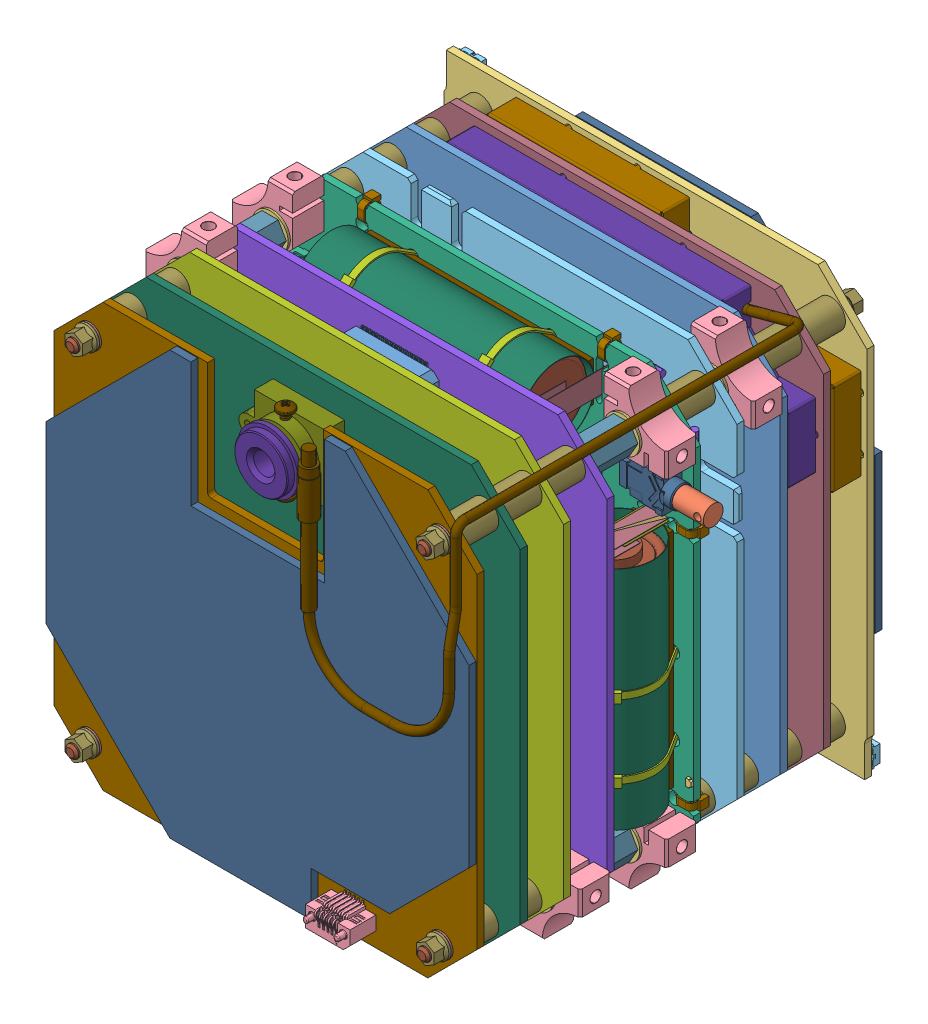
SolidWorks assembly PCB-Stack, configuration Default. Lengths in mm.
Overall size (103.5 98 104.43).
259 component instances, 59 part files, 0 mates.
Components (placement in the parent):
- PCB-Stack.iam-1: PCB-Stack.iam [Default] at origin size (103.5 98 104.43)
  - PCB_TX.iam-1: PCB_TX.iam [Default] at origin size (95 95 16.51)
    - Samtec_QTH-030-02-L-D-A.ipt-1: Samtec_QTH-030-02-L-D-A.ipt [Default] at (0 -31.9938 1.8415) x (0 1 0) z (1 0 0) size (20 8 7.11)
    - Samtec_QSH-030-01-L-D-A.ipt-1: Samtec_QSH-030-01-L-D-A.ipt [Default] at (0 -31.9936 -0.127) x (0 -1 0) z (1 0 0) size (21.31 4 7.49)
    - PCB_TX.ipt-1: PCB_TX.ipt [Default] at origin size (95 95 1.59)
    - Samtec_FSI-105-06-L-S-AD.ipt-1: Samtec_FSI-105-06-L-S-AD.ipt [Default] at (-15 -42.5 -0.2) x (1 0 0) z (0 1 0) size (10 8.86 5.87)
    - C&K_HDT0004.iam-1: C&K_HDT0004.iam [Default] at (44.25 -44.5 0) x (1 0 0) z (0 1 0) size (4.99 3.82 4.7)
      - C&K_HDT0004.ipt-1: C&K_HDT0004.ipt [Default] at origin size (4.9 2.3 4.7)
      - C&K_HDT0004_blade.ipt-1: C&K_HDT0004_blade.ipt [Default] at (0.0272 0.0212 0) x (0.999834 0.018233 0) z (0 0 1) size (2.26 1.67 0.7)
      - C&K_HDT0004_blade.ipt-2: C&K_HDT0004_blade.ipt [Default] at (-0.9606 -0.3806 0) x (0.850594 -0.525824 0) z (0 0 1) size (2.26 1.67 0.7)
    - C&K_HDT0004.iam-2: C&K_HDT0004.iam [Default] at (-44.25 44.5 0) x (-1 0 0) z (0 -1 0) size (4.99 3.82 4.7)
      - C&K_HDT0004.ipt-1: C&K_HDT0004.ipt [Default] at origin size (4.9 2.3 4.7)
      - C&K_HDT0004_blade.ipt-1: C&K_HDT0004_blade.ipt [Default] at (0.0272 0.0212 0) x (0.999834 0.018233 0) z (0 0 1) size (2.26 1.67 0.7)
      - C&K_HDT0004_blade.ipt-2: C&K_HDT0004_blade.ipt [Default] at (-0.9606 -0.3806 0) x (0.850594 -0.525824 0) z (0 0 1) size (2.26 1.67 0.7)
    - Tantalum_4x9x1.ipt-1: Tantalum_4x9x1.ipt [Default] at (10.5 -13.5 3.8375) x (0 1 0) z (0 0 1) size (8.75 4 1)
    - Tantalum_5x7x1.ipt-1: Tantalum_5x7x1.ipt [Default] at (-24 20.25 4.0875) x (-1 0 0) z (0 0 1) size (7 5 1)
    - tx_v2_04_cu_shield.ipt-1: tx_v2_04_cu_shield.ipt [Default] at (-0.2089 -0.202 7.5561) size (77.88 35.38 7.85)
    - Pb_TX_bot.ipt-1: Pb_TX_bot.ipt [Default] at (0 0 -0.9874) size (95 82 1.57)
    - coax_tx.ipt-1: coax_tx.ipt [Default] at (42 22.5 -0.9) x (-1 0 0) z (0 0 -1) size (40.9 68.4 4.41)
  - standoff815mm.ipt-1: standoff815mm.ipt [Default] at (-39.5 -39.5 5.6625) size (6.35 6.35 8.15)
  - standoff815mm.ipt-2: standoff815mm.ipt [Default] at (-39.5 39.5 5.6625) size (6.35 6.35 8.15)
  - standoff815mm.ipt-3: standoff815mm.ipt [Default] at (39.5 39.5 5.6625) size (6.35 6.35 8.15)
  - standoff815mm.ipt-4: standoff815mm.ipt [Default] at (39.5 -39.5 5.6625) size (6.35 6.35 8.15)
  - standoff815mm.ipt-5: standoff815mm.ipt [Default] at (-39.5 -39.5 15.4) size (6.35 6.35 8.15)
  - standoff815mm.ipt-6: standoff815mm.ipt [Default] at (-39.5 39.5 15.4) size (6.35 6.35 8.15)
  - standoff815mm.ipt-7: standoff815mm.ipt [Default] at (39.5 39.5 15.4) size (6.35 6.35 8.15)
  - standoff815mm.ipt-8: standoff815mm.ipt [Default] at (39.5 -39.5 15.4) size (6.35 6.35 8.15)
  - standoff815mm.ipt-9: standoff815mm.ipt [Default] at (-39.5 39.5 25.1375) size (6.35 6.35 8.15)
  - standoff815mm.ipt-10: standoff815mm.ipt [Default] at (39.5 -39.5 25.1375) size (6.35 6.35 8.15)
  - standoff815mm.ipt-11: standoff815mm.ipt [Default] at (-39.5 -39.5 34.875) size (6.35 6.35 8.15)
  - standoff815mm.ipt-12: standoff815mm.ipt [Default] at (-39.5 39.5 34.875) size (6.35 6.35 8.15)
  - standoff815mm.ipt-13: standoff815mm.ipt [Default] at (39.5 39.5 34.875) size (6.35 6.35 8.15)
  - standoff815mm.ipt-14: standoff815mm.ipt [Default] at (39.5 -39.5 34.875) size (6.35 6.35 8.15)
  - standoff815mm.ipt-15: standoff815mm.ipt [Default] at (-39.5 -39.5 64.0875) size (6.35 6.35 8.15)
  - standoff815mm.ipt-16: standoff815mm.ipt [Default] at (39.5 39.5 64.0875) size (6.35 6.35 8.15)
  - standoff815mm.ipt-17: standoff815mm.ipt [Default] at (-39.5 -39.5 73.825) size (6.35 6.35 8.15)
  - standoff815mm.ipt-18: standoff815mm.ipt [Default] at (-39.5 39.5 73.825) size (6.35 6.35 8.15)
  - standoff815mm.ipt-19: standoff815mm.ipt [Default] at (39.5 39.5 73.825) size (6.35 6.35 8.15)
  - standoff815mm.ipt-20: standoff815mm.ipt [Default] at (39.5 -39.5 73.825) size (6.35 6.35 8.15)
  - standoff815mm.ipt-21: standoff815mm.ipt [Default] at (-39.5 -39.5 83.5625) size (6.35 6.35 8.15)
  - standoff815mm.ipt-22: standoff815mm.ipt [Default] at (-39.5 39.5 83.5625) size (6.35 6.35 8.15)
  - standoff815mm.ipt-23: standoff815mm.ipt [Default] at (39.5 39.5 83.5625) size (6.35 6.35 8.15)
  - standoff815mm.ipt-24: standoff815mm.ipt [Default] at (39.5 -39.5 83.5625) size (6.35 6.35 8.15)
  - PCB_RX.iam-1: PCB_RX.iam [Default] at (0 0 9.7375) size (95 95 87.7)
    - Samtec_QSH-030-01-L-D-A.ipt-1: Samtec_QSH-030-01-L-D-A.ipt [Default] at (0 -31.9936 -0.127) x (0 -1 0) z (1 0 0) size (21.31 4 7.49)
    - Samtec_QTH-030-02-L-D-A.ipt-1: Samtec_QTH-030-02-L-D-A.ipt [Default] at (0 -31.9938 1.8415) x (0 1 0) z (1 0 0) size (20 8 7.11)
    - PCB_RX.ipt-1: PCB_RX.ipt [Default] at origin size (95 95 1.59)
    - RX_tan_U7_MBC13917.ipt-1: RX_tan_U7_MBC13917.ipt [Default] at (4.5 42.03 -1) x (-1 0 0) z (0 0 1) size (6.35 6.35 1)
    - RX_tan_U9_SA601.ipt-1: RX_tan_U9_SA601.ipt [Default] at (-23.16 37.32 -1) x (-1 0 0) z (0 0 1) size (6.35 6.35 1)
    - RX_tan_U10_SA607.ipt-1: RX_tan_U10_SA607.ipt [Default] at (-18 4 -1) x (-1 0 0) z (0 0 1) size (6.35 6.35 1)
    - rx_v1_23_cu_shield.ipt-1: rx_v1_23_cu_shield.ipt [Default] at (0 0 7.5565) size (91.38 65.38 7.85)
    - rx_coax.ipt-1: rx_coax.ipt [Default] at (25.5 41.6 2.6035) x (1 0 0) z (0 -1 0) size (34.34 82.88 45.77)
  - PCB_IHU.iam-1: PCB_IHU.iam [Default] at (0 0 19.475) size (95 95 12.08)
    - Samtec_QSH-030-01-L-D-A.ipt-1: Samtec_QSH-030-01-L-D-A.ipt [Default] at (0 -31.9936 -0.127) x (0 -1 0) z (1 0 0) size (21.31 4 7.49)
    - Samtec_QTH-030-02-L-D-A.ipt-1: Samtec_QTH-030-02-L-D-A.ipt [Default] at (0 -31.9938 1.8415) x (0 1 0) z (1 0 0) size (20 8 7.11)
    - PCB_IHU.ipt-1: PCB_IHU.ipt [Default] at origin size (95 95 1.59)
  - spacer_copper.ipt-1: spacer_copper.ipt [Default] at (-39.5 -39.5 25.1375) size (4.76 4.76 8.15)
  - spacer_copper.ipt-2: spacer_copper.ipt [Default] at (39.5 39.5 25.1375) size (4.76 4.76 8.15)
  - spacer_copper.ipt-3: spacer_copper.ipt [Default] at (-39.5 -39.5 44.6125) size (4.76 4.76 8.15)
  - spacer_copper.ipt-4: spacer_copper.ipt [Default] at (-39.5 39.5 44.6125) size (4.76 4.76 8.15)
  - spacer_copper.ipt-5: spacer_copper.ipt [Default] at (39.5 39.5 44.6125) size (4.76 4.76 8.15)
  - spacer_copper.ipt-6: spacer_copper.ipt [Default] at (39.5 -39.5 44.6125) size (4.76 4.76 8.15)
  - spacer_copper.ipt-7: spacer_copper.ipt [Default] at (39.5 -39.5 55.9375) x (0.997727 -0.067389 0) z (0 0 -1) size (4.76 4.76 8.15)
  - spacer_copper.ipt-8: spacer_copper.ipt [Default] at (-39.5 39.5 55.9375) x (1 0 0) z (0 0 -1) size (4.76 4.76 8.15)
  - 90792A312_shimwasher.ipt-1: 90792A312_shimwasher.ipt [Default] at (-39.5 -39.5 21.0625) size (7.95 7.95 0.25)
  - 90792A312_shimwasher.ipt-2: 90792A312_shimwasher.ipt [Default] at (39.5 39.5 21.0625) size (7.95 7.95 0.25)
  - 90792A312_shimwasher.ipt-3: 90792A312_shimwasher.ipt [Default] at (-39.5 -39.5 28.6375) size (7.95 7.95 0.25)
  - 90792A312_shimwasher.ipt-4: 90792A312_shimwasher.ipt [Default] at (39.5 39.5 28.6375) size (7.95 7.95 0.25)
  - 90792A312_shimwasher.ipt-5: 90792A312_shimwasher.ipt [Default] at (-39.5 -39.5 40.5375) size (7.95 7.95 0.25)
  - 90792A312_shimwasher.ipt-6: 90792A312_shimwasher.ipt [Default] at (-39.5 -39.5 48.1125) size (7.95 7.95 0.25)
  - 90792A312_shimwasher.ipt-7: 90792A312_shimwasher.ipt [Default] at (-39.5 39.5 40.5375) size (7.95 7.95 0.25)
  - 90792A312_shimwasher.ipt-8: 90792A312_shimwasher.ipt [Default] at (-39.5 39.5 48.1125) size (7.95 7.95 0.25)
  - 90792A312_shimwasher.ipt-9: 90792A312_shimwasher.ipt [Default] at (39.5 39.5 40.5375) size (7.95 7.95 0.25)
  - 90792A312_shimwasher.ipt-10: 90792A312_shimwasher.ipt [Default] at (39.5 39.5 48.1125) size (7.95 7.95 0.25)
  - 90792A312_shimwasher.ipt-11: 90792A312_shimwasher.ipt [Default] at (39.5 -39.5 40.5375) size (7.95 7.95 0.25)
  - 90792A312_shimwasher.ipt-12: 90792A312_shimwasher.ipt [Default] at (39.5 -39.5 48.1125) size (7.95 7.95 0.25)
  - 90792A312_shimwasher.ipt-13: 90792A312_shimwasher.ipt [Default] at (-39.5 39.5 60.0125) size (7.95 7.95 0.25)
  - 90792A312_shimwasher.ipt-14: 90792A312_shimwasher.ipt [Default] at (-39.5 39.5 60.2665) size (7.95 7.95 0.25)
  - 90792A312_shimwasher.ipt-15: 90792A312_shimwasher.ipt [Default] at (39.5 -39.5 60.0125) size (7.95 7.95 0.25)
  - 90792A312_shimwasher.ipt-16: 90792A312_shimwasher.ipt [Default] at (39.5 -39.5 60.2665) size (7.95 7.95 0.25)
  - 90792A312_shimwasher.ipt-17: 90792A312_shimwasher.ipt [Default] at (-39.5 39.5 67.5205) size (7.95 7.95 0.25)
  - 90792A312_shimwasher.ipt-18: 90792A312_shimwasher.ipt [Default] at (-39.5 39.5 67.7745) size (7.95 7.95 0.25)
  - 90792A312_shimwasher.ipt-19: 90792A312_shimwasher.ipt [Default] at (39.5 -39.5 67.5205) size (7.95 7.95 0.25)
  - 90792A312_shimwasher.ipt-20: 90792A312_shimwasher.ipt [Default] at (39.5 -39.5 67.7745) size (7.95 7.95 0.25)
  - 90792A312_shimwasher.ipt-21: 90792A312_shimwasher.ipt [Default] at (-39.5 -39.5 21.3165) size (7.95 7.95 0.25)
  - 90792A312_shimwasher.ipt-22: 90792A312_shimwasher.ipt [Default] at (39.5 39.5 21.3165) size (7.95 7.95 0.25)
  - 90792A312_shimwasher.ipt-23: 90792A312_shimwasher.ipt [Default] at (-39.5 -39.5 28.8915) size (7.95 7.95 0.25)
  - 90792A312_shimwasher.ipt-24: 90792A312_shimwasher.ipt [Default] at (39.5 39.5 28.8915) size (7.95 7.95 0.25)
  - 90792A312_shimwasher.ipt-25: 90792A312_shimwasher.ipt [Default] at (39.5 -39.5 40.7915) size (7.95 7.95 0.25)
  - 90792A312_shimwasher.ipt-26: 90792A312_shimwasher.ipt [Default] at (-39.5 -39.5 40.7915) size (7.95 7.95 0.25)
  - 90792A312_shimwasher.ipt-27: 90792A312_shimwasher.ipt [Default] at (39.5 39.5 40.7915) size (7.95 7.95 0.25)
  - 90792A312_shimwasher.ipt-28: 90792A312_shimwasher.ipt [Default] at (-39.5 39.5 40.7915) size (7.95 7.95 0.25)
  - 90792A312_shimwasher.ipt-29: 90792A312_shimwasher.ipt [Default] at (-39.5 39.5 48.3665) size (7.95 7.95 0.25)
  - 90792A312_shimwasher.ipt-30: 90792A312_shimwasher.ipt [Default] at (-39.5 -39.5 48.3665) size (7.95 7.95 0.25)
  - 90792A312_shimwasher.ipt-31: 90792A312_shimwasher.ipt [Default] at (39.5 -39.5 48.3665) size (7.95 7.95 0.25)
  - 90792A312_shimwasher.ipt-32: 90792A312_shimwasher.ipt [Default] at (39.5 39.5 48.3665) size (7.95 7.95 0.25)
  - delrin_pcb_mount4.ipt-1: delrin_pcb_mount4.ipt [Default] at (49 49 25.1375) x (-1 0 0) z (0 0 1) size (14 14 7)
  - delrin_pcb_mount4.ipt-2: delrin_pcb_mount4.ipt [Default] at (-49 49 44.6125) x (0 -1 0) z (0 0 1) size (14 14 7)
  - delrin_pcb_mount4.ipt-3: delrin_pcb_mount4.ipt [Default] at (49 49 44.6125) x (-1 0 0) z (0 0 1) size (14 14 7)
  - delrin_pcb_mount4.ipt-4: delrin_pcb_mount4.ipt [Default] at (49 -49 44.6125) x (0 1 0) z (0 0 1) size (14 14 7)
  - delrin_pcb_mount4.ipt-5: delrin_pcb_mount4.ipt [Default] at (-49 49 64.0205) x (0 -1 0) z (0 0 1) size (14 14 7)
  - delrin_pcb_mount4.ipt-6: delrin_pcb_mount4.ipt [Default] at (49 -49 64.0205) x (0 1 0) z (0 0 1) size (14 14 7)
  - PCB_PSU.iam-1: PCB_PSU.iam [Default] at (0 0 29.2125) size (95 95 12.08)
    - Samtec_QSH-030-01-L-D-A.ipt-1: Samtec_QSH-030-01-L-D-A.ipt [Default] at (0 -31.9936 -0.127) x (0 -1 0) z (1 0 0) size (21.31 4 7.49)
    - Samtec_QTH-030-02-L-D-A.ipt-1: Samtec_QTH-030-02-L-D-A.ipt [Default] at (0 -31.9938 1.8415) x (0 1 0) z (1 0 0) size (20 8 7.11)
    - PCB_PSU.ipt-1: PCB_PSU.ipt [Default] at origin size (95 95 1.59)
  - battery6A.iam-1: battery6A.iam [Default] at (0 0 44.5375) size (95.25 95.25 22.75)
    - PCB_Batt1.iam-1: PCB_Batt1.iam [Default] at (0 0 -5.5875) size (95 95 12.08)
      - PCB_Batt1.ipt-1: PCB_Batt1.ipt [Default] at origin size (95 95 1.59)
      - Samtec_QSH-030-01-L-D-A.ipt-1: Samtec_QSH-030-01-L-D-A.ipt [Default] at (0 -31.9936 -0.127) x (0 -1 0) z (1 0 0) size (21.31 4 7.49)
      - Samtec_QTH-030-02-L-D-A.ipt-1: Samtec_QTH-030-02-L-D-A.ipt [Default] at (0 -31.9938 1.8415) x (0 1 0) z (1 0 0) size (20 8 7.11)
    - battery_cord_2x.ipt-1: battery_cord_2x.ipt [Default] at (30.1001 -22 -5.95) x (0 1 0) z (1 0 0) size (2 19.3 34.3)
    - battery_cord_2x.ipt-2: battery_cord_2x.ipt [Default] at (30 -5.6143 -5.95) x (0 1 0) z (1 0 0) size (2 19.3 34.3)
    - battery_cord_2x.ipt-3: battery_cord_2x.ipt [Default] at (-30.1001 -22 -5.95) x (0 -1 0) z (-1 0 0) size (2 19.3 34.3)
    - battery_cord_2x.ipt-4: battery_cord_2x.ipt [Default] at (-30 -5.6143 -5.95) x (0 -1 0) z (-1 0 0) size (2 19.3 34.3)
    - battery_cord_2x.ipt-5: battery_cord_2x.ipt [Default] at (15.5 30.1001 -5.95) x (-1 0 0) z (0 1 0) size (2 19.3 34.3)
    - battery_cord_2x.ipt-6: battery_cord_2x.ipt [Default] at (-15.5 30.1001 -5.95) x (-1 0 0) z (0 1 0) size (2 19.3 34.3)
    - hysteresis_rod.ipt-1: hysteresis_rod.ipt [Default] at (45.25 0 -6.4003) x (0 0 1) z (0 1 0) size (1.57 1.57 76.2)
    - hysteresis_rod.ipt-2: hysteresis_rod.ipt [Default] at (0 45.25 -6.4003) x (0 0 1) z (-1 0 0) size (1.57 1.57 76.2)
    - hysteresis_cord.ipt-1: hysteresis_cord.ipt [Default] at (45.25 -33.45 -3.85) x (0 -1 0) z (1 0 0) size (2 3.9 4.45)
    - hysteresis_cord.ipt-2: hysteresis_cord.ipt [Default] at (45.25 19.55 -3.85) x (0 -1 0) z (1 0 0) size (2 3.9 4.45)
    - hysteresis_cord.ipt-3: hysteresis_cord.ipt [Default] at (27 45.25 -3.85) x (1 0 0) z (0 1 0) size (2 3.9 4.45)
    - hysteresis_cord.ipt-4: hysteresis_cord.ipt [Default] at (-27 45.25 -3.85) x (1 0 0) z (0 1 0) size (2 3.9 4.45)
    - CUI_audio_SJ1-42536-SMT.ipt-1: CUI_audio_SJ1-42536-SMT.ipt [Default] at (45 28.5 -1.42) x (1 0 0) z (0 -1 0) size (12.5 5.6 10.4)
    - battery_A_SanyoKR1700AU.iam-1: battery_A_SanyoKR1700AU.iam [Default] at (-38.5 -6.5 4.45) x (0 0 1) z (0 -1 0) size (22.45 16.9 51.9)
      - battery_A_SanyoKR1700AU.ipt-1: battery_A_SanyoKR1700AU.ipt [Default] at origin size (16.5 16.5 48.5)
      - battery_tab_straight.ipt-1: battery_tab_straight.ipt [Default] at (0 0 -24.35) x (0 0 -1) z (0 -1 0) size (1.7 17.85 5)
      - battery_tab_straight.ipt-2: battery_tab_straight.ipt [Default] at (0 0 24.35) x (0 0 1) z (0 1 0) size (1.7 17.85 5)
      - battery_tab_folded.ipt-1: battery_tab_folded.ipt [Default] at (0 0 -24.35) x (0 0 -1) z (0 -1 0) size (3.6 14.15 5)
      - battery_tab_folded.ipt-2: battery_tab_folded.ipt [Default] at (0 0 24.35) x (0 0 1) z (0 1 0) size (3.6 14.15 5)
      - kaptonheater_OmegaKHLV102.ipt-1: kaptonheater_OmegaKHLV102.ipt [Default] at origin size (14.25 14.25 50)
      - kapton_wrap_battery.ipt-1: kapton_wrap_battery.ipt [Default] at origin size (16.9 16.9 50.8)
      - kapton_battery_tab.ipt-1: kapton_battery_tab.ipt [Default] at (-4 0 25.75) x (0 -1 0) z (0 0 1) size (6 10 0.1)
    - battery_A_SanyoKR1700AU.iam-2: battery_A_SanyoKR1700AU.iam [Default] at (-21.6 -21.1143 4.45) x (0 0 1) z (0 -1 0) size (22.45 16.9 51.9)
      - battery_A_SanyoKR1700AU.ipt-1: battery_A_SanyoKR1700AU.ipt [Default] at origin size (16.5 16.5 48.5)
      - battery_tab_straight.ipt-1: battery_tab_straight.ipt [Default] at (0 0 -24.35) x (0 0 -1) z (0 -1 0) size (1.7 17.85 5)
      - battery_tab_straight.ipt-2: battery_tab_straight.ipt [Default] at (0 0 24.35) x (0 0 1) z (0 1 0) size (1.7 17.85 5)
      - battery_tab_folded.ipt-1: battery_tab_folded.ipt [Default] at (0 0 -24.35) x (0 0 -1) z (0 -1 0) size (3.6 14.15 5)
      - battery_tab_folded.ipt-2: battery_tab_folded.ipt [Default] at (0 0 24.35) x (0 0 1) z (0 1 0) size (3.6 14.15 5)
      - kaptonheater_OmegaKHLV102.ipt-1: kaptonheater_OmegaKHLV102.ipt [Default] at origin size (14.25 14.25 50)
      - kapton_wrap_battery.ipt-1: kapton_wrap_battery.ipt [Default] at origin size (16.9 16.9 50.8)
      - kapton_battery_tab.ipt-1: kapton_battery_tab.ipt [Default] at (-4 0 25.75) x (0 -1 0) z (0 0 1) size (6 10 0.1)
    - battery_A_SanyoKR1700AU.iam-3: battery_A_SanyoKR1700AU.iam [Default] at (0 38.5 4.45) x (0 0 1) z (-1 0 0) size (22.45 16.9 51.9)
      - battery_A_SanyoKR1700AU.ipt-1: battery_A_SanyoKR1700AU.ipt [Default] at origin size (16.5 16.5 48.5)
      - battery_tab_straight.ipt-1: battery_tab_straight.ipt [Default] at (0 0 -24.35) x (0 0 -1) z (0 -1 0) size (1.7 17.85 5)
      - battery_tab_straight.ipt-2: battery_tab_straight.ipt [Default] at (0 0 24.35) x (0 0 1) z (0 1 0) size (1.7 17.85 5)
      - battery_tab_folded.ipt-1: battery_tab_folded.ipt [Default] at (0 0 -24.35) x (0 0 -1) z (0 -1 0) size (3.6 14.15 5)
      - battery_tab_folded.ipt-2: battery_tab_folded.ipt [Default] at (0 0 24.35) x (0 0 1) z (0 1 0) size (3.6 14.15 5)
      - kaptonheater_OmegaKHLV102.ipt-1: kaptonheater_OmegaKHLV102.ipt [Default] at origin size (14.25 14.25 50)
      - kapton_wrap_battery.ipt-1: kapton_wrap_battery.ipt [Default] at origin size (16.9 16.9 50.8)
      - kapton_battery_tab.ipt-1: kapton_battery_tab.ipt [Default] at (-4 0 25.75) x (0 -1 0) z (0 0 1) size (6 10 0.1)
    - battery_A_SanyoKR1700AU.iam-4: battery_A_SanyoKR1700AU.iam [Default] at (0 21.6 4.45) x (0 0 1) z (-1 0 0) size (22.45 16.9 51.9)
      - battery_A_SanyoKR1700AU.ipt-1: battery_A_SanyoKR1700AU.ipt [Default] at origin size (16.5 16.5 48.5)
      - battery_tab_straight.ipt-1: battery_tab_straight.ipt [Default] at (0 0 -24.35) x (0 0 -1) z (0 -1 0) size (1.7 17.85 5)
      - battery_tab_straight.ipt-2: battery_tab_straight.ipt [Default] at (0 0 24.35) x (0 0 1) z (0 1 0) size (1.7 17.85 5)
      - battery_tab_folded.ipt-1: battery_tab_folded.ipt [Default] at (0 0 -24.35) x (0 0 -1) z (0 -1 0) size (3.6 14.15 5)
      - battery_tab_folded.ipt-2: battery_tab_folded.ipt [Default] at (0 0 24.35) x (0 0 1) z (0 1 0) size (3.6 14.15 5)
      - kaptonheater_OmegaKHLV102.ipt-1: kaptonheater_OmegaKHLV102.ipt [Default] at origin size (14.25 14.25 50)
      - kapton_wrap_battery.ipt-1: kapton_wrap_battery.ipt [Default] at origin size (16.9 16.9 50.8)
      - kapton_battery_tab.ipt-1: kapton_battery_tab.ipt [Default] at (-4 0 25.75) x (0 -1 0) z (0 0 1) size (6 10 0.1)
    - battery_A_SanyoKR1700AU.iam-5: battery_A_SanyoKR1700AU.iam [Default] at (21.6 -21.1143 4.45) x (0 0 1) z (0 1 0) size (22.45 16.9 51.9)
      - battery_A_SanyoKR1700AU.ipt-1: battery_A_SanyoKR1700AU.ipt [Default] at origin size (16.5 16.5 48.5)
      - battery_tab_straight.ipt-1: battery_tab_straight.ipt [Default] at (0 0 -24.35) x (0 0 -1) z (0 -1 0) size (1.7 17.85 5)
      - battery_tab_straight.ipt-2: battery_tab_straight.ipt [Default] at (0 0 24.35) x (0 0 1) z (0 1 0) size (1.7 17.85 5)
      - battery_tab_folded.ipt-1: battery_tab_folded.ipt [Default] at (0 0 -24.35) x (0 0 -1) z (0 -1 0) size (3.6 14.15 5)
      - battery_tab_folded.ipt-2: battery_tab_folded.ipt [Default] at (0 0 24.35) x (0 0 1) z (0 1 0) size (3.6 14.15 5)
      - kaptonheater_OmegaKHLV102.ipt-1: kaptonheater_OmegaKHLV102.ipt [Default] at origin size (14.25 14.25 50)
      - kapton_wrap_battery.ipt-1: kapton_wrap_battery.ipt [Default] at origin size (16.9 16.9 50.8)
      - kapton_battery_tab.ipt-1: kapton_battery_tab.ipt [Default] at (-4 0 25.75) x (0 -1 0) z (0 0 1) size (6 10 0.1)
    - battery_A_SanyoKR1700AU.iam-6: battery_A_SanyoKR1700AU.iam [Default] at (38.5 -6.5 4.45) x (0 0 1) z (0 1 0) size (22.45 16.9 51.9)
      - battery_A_SanyoKR1700AU.ipt-1: battery_A_SanyoKR1700AU.ipt [Default] at origin size (16.5 16.5 48.5)
      - battery_tab_straight.ipt-1: battery_tab_straight.ipt [Default] at (0 0 -24.35) x (0 0 -1) z (0 -1 0) size (1.7 17.85 5)
      - battery_tab_straight.ipt-2: battery_tab_straight.ipt [Default] at (0 0 24.35) x (0 0 1) z (0 1 0) size (1.7 17.85 5)
      - battery_tab_folded.ipt-1: battery_tab_folded.ipt [Default] at (0 0 -24.35) x (0 0 -1) z (0 -1 0) size (3.6 14.15 5)
      - battery_tab_folded.ipt-2: battery_tab_folded.ipt [Default] at (0 0 24.35) x (0 0 1) z (0 1 0) size (3.6 14.15 5)
      - kaptonheater_OmegaKHLV102.ipt-1: kaptonheater_OmegaKHLV102.ipt [Default] at origin size (14.25 14.25 50)
      - kapton_wrap_battery.ipt-1: kapton_wrap_battery.ipt [Default] at origin size (16.9 16.9 50.8)
      - kapton_battery_tab.ipt-1: kapton_battery_tab.ipt [Default] at (-4 0 25.75) x (0 -1 0) z (0 0 1) size (6 10 0.1)
    - signal_relay_panasonic_tx.ipt-1: signal_relay_panasonic_tx.ipt [Default] at (4.5 3.5 0.1) x (1 0 0) z (0 -1 0) size (15 8.2 7.4)
    - signal_relay_panasonic_tx.ipt-2: signal_relay_panasonic_tx.ipt [Default] at (-8 -5 0.1) x (0 1 0) z (-1 0 0) size (15 8.2 7.4)
    - epoxy_under-battery.ipt-1: epoxy_under-battery.ipt [Default] at (-38.5 -6.5 -4) x (-1 0 0) z (0 1 0) size (9 1.35 50)
    - epoxy_under-battery.ipt-2: epoxy_under-battery.ipt [Default] at (-21.6 -21.1143 -4) x (1 0 0) z (0 -1 0) size (9 1.35 50)
    - epoxy_under-battery.ipt-3: epoxy_under-battery.ipt [Default] at (0 38.5 -4) x (0 -1 0) z (-1 0 0) size (9 1.35 50)
    - epoxy_under-battery.ipt-4: epoxy_under-battery.ipt [Default] at (0 21.6 -4) x (0 -1 0) z (-1 0 0) size (9 1.35 50)
    - epoxy_under-battery.ipt-5: epoxy_under-battery.ipt [Default] at (21.6 -21.1143 -4) x (-1 0 0) z (0 1 0) size (9 1.35 50)
    - epoxy_under-battery.ipt-6: epoxy_under-battery.ipt [Default] at (38.5 -6.5 -4) x (-1 0 0) z (0 1 0) size (9 1.35 50)
    - epoxy_under-battery.ipt-7: epoxy_under-battery.ipt [Default] at (0 30 4.45) x (0 0 -1) z (1 0 0) size (9 1.35 50)
    - epoxy_under-battery.ipt-8: epoxy_under-battery.ipt [Default] at (0 30.1 4.45) x (0 0 -1) z (-1 0 0) size (9 1.35 50)
    - epoxy_under-battery_short.ipt-1: epoxy_under-battery_short.ipt [Default] at (-30 -13.45 4.45) x (0 0 -1) z (0 1 0) size (9 1.35 34.4)
    - epoxy_under-battery_short.ipt-2: epoxy_under-battery_short.ipt [Default] at (-30.1 -14.0643 4.45) x (0 0 -1) z (0 -1 0) size (9 1.35 34.4)
    - epoxy_under-battery_short.ipt-3: epoxy_under-battery_short.ipt [Default] at (30.1 -14.1643 4.45) x (0 0 -1) z (0 1 0) size (9 1.35 34.4)
    - epoxy_under-battery_short.ipt-4: epoxy_under-battery_short.ipt [Default] at (30 -13.55 4.45) x (0 0 -1) z (0 -1 0) size (9 1.35 34.4)
    - thermistor_batteries.ipt-1: thermistor_batteries.ipt [Default] at (-30.05 -14.11 8.95) x (-1 0 0) z (0 -1 0) size (2.29 2.29 20.08)
    - thermistor_batteries.ipt-2: thermistor_batteries.ipt [Default] at (30 -14.21 8.95) x (-1 0 0) z (0 -1 0) size (2.29 2.29 20.08)
    - thermistor_batteries.ipt-3: thermistor_batteries.ipt [Default] at (0 30 8.95) x (0 -1 0) z (1 0 0) size (2.29 2.29 20.08)
    - LED_LTST-S270KFKT.ipt-1: LED_LTST-S270KFKT.ipt [Default] at (-46.35 -28.5 -3.7) size (1.15 1.65 0.6)
    - LED_LTST-S270KFKT.ipt-2: LED_LTST-S270KFKT.ipt [Default] at (46.35 -28.5 -3.7) x (-1 0 0) z (0 0 -1) size (1.15 1.65 0.6)
    - shielded_power_inductor_CC1360.ipt-1: shielded_power_inductor_CC1360.ipt [Default] at (6 -13.5 -3.1) x (0 -1 0) z (0 0 1) size (12.7 12.6 5.45)
    - piezo_sounder_PKLCS.ipt-1: piezo_sounder_PKLCS.ipt [Default] at (-7.5 -13.5 -2.5) x (0 1 0) z (0 0 1) size (12 12 3)
    - MiniUSB-B_Molex548190519.ipt-1: MiniUSB-B_Molex548190519.ipt [Default] at (-47.5 28 -2) x (0 -1 0) z (-1 0 0) size (7.7 5.76 9)
  - PCB_Exp2.iam-1: PCB_Exp2.iam [Default] at (0 0 68.1625) size (95 95 12.08)
    - Samtec_QSH-030-01-L-D-A.ipt-1: Samtec_QSH-030-01-L-D-A.ipt [Default] at (0 -31.9936 -0.127) x (0 -1 0) z (1 0 0) size (21.31 4 7.49)
    - Samtec_QSH-030-01-L-D-A.ipt-2: Samtec_QSH-030-01-L-D-A.ipt [Default] at (0 39.5 -0.127) x (-1 0 0) z (0 -1 0) size (21.31 4 7.49)
    - Samtec_QTH-030-02-L-D-A.ipt-1: Samtec_QTH-030-02-L-D-A.ipt [Default] at (0 -31.9938 1.8415) x (0 1 0) z (1 0 0) size (20 8 7.11)
    - PCB_Exp2.ipt-1: PCB_Exp2.ipt [Default] at origin size (95 95 1.59)
  - PCB_Exp1.iam-1: PCB_Exp1.iam [Default] at (0 0 58.425) size (95 95 12.08)
    - Samtec_QSH-030-01-L-D-A.ipt-1: Samtec_QSH-030-01-L-D-A.ipt [Default] at (0 -31.9936 -0.127) x (0 -1 0) z (1 0 0) size (21.31 4 7.49)
    - Samtec_QTH-030-02-L-D-A.ipt-1: Samtec_QTH-030-02-L-D-A.ipt [Default] at (0 -31.9938 1.8415) x (0 1 0) z (1 0 0) size (20 8 7.11)
    - Samtec_QTH-030-02-L-D-A.ipt-2: Samtec_QTH-030-02-L-D-A.ipt [Default] at (0 39.5 1.7907) x (1 0 0) z (0 -1 0) size (20 8 7.11)
    - PCB_Exp1.ipt-1: PCB_Exp1.ipt [Default] at origin size (95 95 1.59)
  - PCB_Exp4.iam-1: PCB_Exp4.iam [Default] at (0 0 87.6375) size (95 95 12.37)
    - Samtec_QSH-030-01-L-D-A.ipt-1: Samtec_QSH-030-01-L-D-A.ipt [Default] at (0 -31.9936 -0.127) x (0 -1 0) z (1 0 0) size (21.31 4 7.49)
    - PCB_Exp4.ipt-1: PCB_Exp4.ipt [Default] at origin size (95 95 1.59)
    - Samtec_FSI-105-06-L-S-AD.ipt-1: Samtec_FSI-105-06-L-S-AD.ipt [Default] at (15 -42.5 1.7875) x (-1 0 0) z (0 1 0) size (10 8.86 5.87)
    - Tant_Exp4_top.ipt-1: Tant_Exp4_top.ipt [Default] at (0 0 2.5749) size (95 95 1.57)
  - threaded_rod.ipt-1: threaded_rod.ipt [Default] at (-39.5 -39.5 44.6125) size (2.84 2.84 98)
  - threaded_rod.ipt-2: threaded_rod.ipt [Default] at (-39.5 39.5 44.6125) size (2.84 2.84 98)
  - threaded_rod.ipt-3: threaded_rod.ipt [Default] at (39.5 -39.5 44.6125) size (2.84 2.84 98)
  - threaded_rod.ipt-4: threaded_rod.ipt [Default] at (39.5 39.5 44.6125) size (2.84 2.84 98)
  - MS21043-04.ipt-1: MS21043-04.ipt [Default] at (-39.5 -39.5 -0.4064) x (1 0 0) z (0 0 -1) size (5.23 5.23 3.17)
  - MS21043-04.ipt-2: MS21043-04.ipt [Default] at (-39.5 39.5 -0.4064) x (1 0 0) z (0 0 -1) size (5.23 5.23 3.17)
  - MS21043-04.ipt-3: MS21043-04.ipt [Default] at (39.5 39.5 -0.4064) x (1 0 0) z (0 0 -1) size (5.23 5.23 3.17)
  - MS21043-04.ipt-4: MS21043-04.ipt [Default] at (39.5 -39.5 -0.4064) x (1 0 0) z (0 0 -1) size (5.23 5.23 3.17)
  - MS21043-04.ipt-5: MS21043-04.ipt [Default] at (-39.5 -39.5 89.6314) size (5.23 5.23 3.17)
  - MS21043-04.ipt-6: MS21043-04.ipt [Default] at (-39.5 39.5 89.6314) size (5.23 5.23 3.17)
  - MS21043-04.ipt-7: MS21043-04.ipt [Default] at (39.5 39.5 89.6314) x (0.997878 0.065108 0) z (0 0 1) size (5.23 5.23 3.17)
  - MS21043-04.ipt-8: MS21043-04.ipt [Default] at (39.5 -39.5 89.6314) size (5.23 5.23 3.17)
  - NAS620-4L.ipt-1: NAS620-4L.ipt [Default] at (-39.5 -39.5 -0.2032) x (1 0 0) z (0 0 -1) size (5.31 5.31 0.41)
  - NAS620-4L.ipt-2: NAS620-4L.ipt [Default] at (-39.5 39.5 -0.2032) x (1 0 0) z (0 0 -1) size (5.31 5.31 0.41)
  - NAS620-4L.ipt-3: NAS620-4L.ipt [Default] at (39.5 39.5 -0.2032) x (1 0 0) z (0 0 -1) size (5.31 5.31 0.41)
  - NAS620-4L.ipt-4: NAS620-4L.ipt [Default] at (39.5 -39.5 -0.2032) x (1 0 0) z (0 0 -1) size (5.31 5.31 0.41)
  - NAS620-4L.ipt-5: NAS620-4L.ipt [Default] at (-39.5 -39.5 89.4282) x (1 0 0) z (0 0 -1) size (5.31 5.31 0.41)
  - NAS620-4L.ipt-6: NAS620-4L.ipt [Default] at (-39.5 39.5 89.4282) x (0.942825 0.333287 0) z (0 0 -1) size (5.31 5.31 0.41)
  - NAS620-4L.ipt-7: NAS620-4L.ipt [Default] at (39.5 -39.5 89.4282) x (0.999994 -0.003425 0) z (0 0 -1) size (5.31 5.31 0.41)
  - NAS620-4L.ipt-8: NAS620-4L.ipt [Default] at (39.5 39.5 89.4282) x (0.997878 0.065108 0) z (0 0 1) size (5.31 5.31 0.41)
  - spacer_threaded.ipt-1: spacer_threaded.ipt [Default] at (-39.5 -39.5 58.4375) x (-0.69952 -0.714613 0) z (0 0 -1) size (7.33 6.35 9.75)
  - spacer_threaded.ipt-2: spacer_threaded.ipt [Default] at (-39.5 39.5 58.4375) x (1 0 0) z (0 0 -1) size (7.33 6.35 9.75)
  - spacer_threaded.ipt-3: spacer_threaded.ipt [Default] at (39.5 39.5 58.4375) x (1 0 0) z (0 0 -1) size (7.33 6.35 9.75)
  - spacer_threaded.ipt-4: spacer_threaded.ipt [Default] at (39.5 -39.5 58.4375) x (1 0 0) z (0 0 -1) size (7.33 6.35 9.75)
  - PCB_Exp3.iam-1: PCB_Exp3.iam [Default] at (0 0 77.9) size (95 95 15.56)
    - Samtec_QSH-030-01-L-D-A.ipt-1: Samtec_QSH-030-01-L-D-A.ipt [Default] at (0 -31.9936 -0.127) x (0 -1 0) z (1 0 0) size (21.31 4 7.49)
    - Samtec_QTH-030-02-L-D-A.ipt-1: Samtec_QTH-030-02-L-D-A.ipt [Default] at (0 -31.9938 1.8415) x (0 1 0) z (1 0 0) size (20 8 7.11)
    - PCB_Exp3.ipt-1: PCB_Exp3.ipt [Default] at origin size (95 95 1.59)
    - cameramount2.ipt-1: cameramount2.ipt [Default] at (-0.0016 34.4901 1.5875) x (0 -1 0) z (-1 0 0) size (15 7.2 23.27)
    - lens.ipt-1: lens.ipt [Default] at (-0.0016 34.4901 9.7875) size (13.5 13.5 6.5)
    - 91772A065_1-72x3-16_pan.ipt-1: 91772A065_1-72x3-16_pan.ipt [Default] at (9.4976 34.4901 4.7625) x (1 0 0) z (0 0 -1) size (3.61 3.61 6.06)
    - 91772A065_1-72x3-16_pan.ipt-2: 91772A065_1-72x3-16_pan.ipt [Default] at (-9.5016 34.4901 4.7625) x (1 0 0) z (0 0 -1) size (3.61 3.61 6.06)
    - 91772A065_1-72x3-16_pan.ipt-3: 91772A065_1-72x3-16_pan.ipt [Default] at (-0.0016 37.7276 6.7875) x (1 0 0) z (0 1 0) size (3.61 3.61 6.06)
    - 91772A065_1-72x3-16_pan.ipt-4: 91772A065_1-72x3-16_pan.ipt [Default] at (-0.0016 31.2526 6.7875) x (-0.84925 0 0.527992) z (0 -1 0) size (3.61 3.61 6.06)
  - PCB_Batt2.iam-1: PCB_Batt2.iam [Default] at (0 0 48.6875) size (16 31 12.08)
    - PCB_Batt2.ipt-1: PCB_Batt2.ipt [Default] at origin size (16 31 1.59)
    - Samtec_QTH-030-02-L-D-A.ipt-1: Samtec_QTH-030-02-L-D-A.ipt [Default] at (0 -31.9938 1.8415) x (0 1 0) z (1 0 0) size (20 8 7.11)
    - Samtec_QSH-030-01-L-D-A.ipt-1: Samtec_QSH-030-01-L-D-A.ipt [Default] at (0 -31.9936 -0.127) x (0 -1 0) z (1 0 0) size (21.31 4 7.49)
  - safe_rbf.ipt-1: safe_rbf.ipt [Default] at (36.5 28.5 43.1175) size (18 4.45 4.46)
  - delrin_pcb_mount4_magnet.ipt-1: delrin_pcb_mount4_magnet.ipt [Default] at (-49 -49 25.1375) size (14 14 7)
  - delrin_pcb_mount4_magnet.ipt-2: delrin_pcb_mount4_magnet.ipt [Default] at (-49 -49 44.6125) x (0 1 0) z (0 0 -1) size (14 14 7)
  - magnet.iam-1: magnet.iam [Default] at (-44.5 -44.5 38.2125) size (6.35 6.35 51.8)
    - magnet.ipt-1: magnet.ipt [Default] at origin size (3.17 3.17 51.8)
    - magnet_spacer.ipt-1: magnet_spacer.ipt [Default] at (0 0 -3.33) size (6.35 6.35 23)
